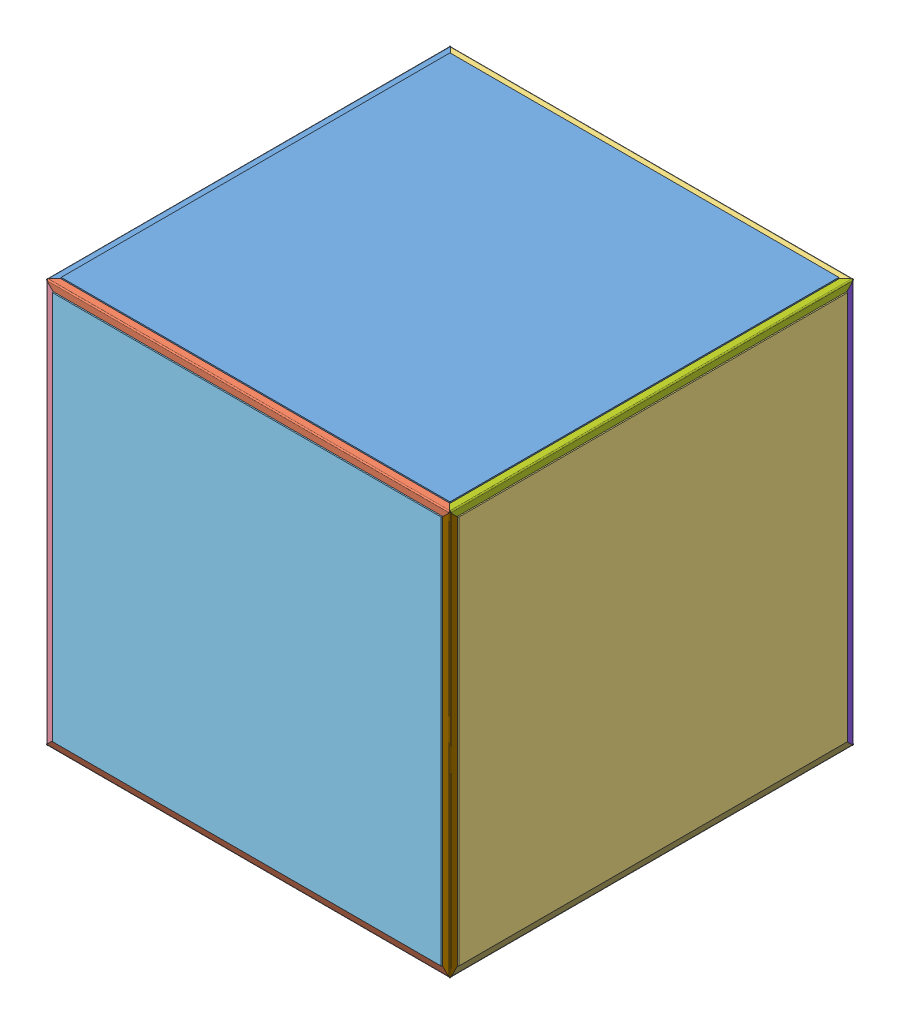
SolidWorks assembly cube_32, configuration cube32. Lengths in mm.
Overall size (513.72 513.72 513.72).
30 component instances, 30 part files, 93 mates.
Components (placement in the parent):
- pr^cube_32-28: pr^cube_32 [cube01] x (-1 0 0) z (0 0 1) size (491.49 1.59 491.49) (virtual)
- pg^cube_32-20: pg^cube_32 [cube01] x (0 -1 0) z (0 0 1) size (491.49 1.59 491.49) (virtual)
- po^cube_32-22: po^cube_32 [cube01] x (0 1 0) z (0 0 1) size (491.49 1.59 491.49) (virtual)
- py^cube_32-21: py^cube_32 [cube01] at origin size (491.49 1.59 491.49) (virtual)
- pc^cube_32-18: pc^cube_32 [cube01] x (-1 0 0) z (0 -1 0) size (491.49 1.59 491.49) (virtual)
- pb^cube_32-21: pb^cube_32 [cube01] x (-1 0 0) z (0 1 0) size (491.49 1.59 491.49) (virtual)
- br1^cube_32-49: br1^cube_32 [Default] at (0 229.87 -229.87) x (0 0 1) z (-1 0 0) size (50.8 50.8 452.63) (virtual)
- br2^cube_32-61: br2^cube_32 [Default] at (-229.87 229.87 0) size (50.8 50.8 452.63) (virtual)
- br3^cube_32-46: br3^cube_32 [Default] at (0 229.87 229.87) x (0 0 -1) z (1 0 0) size (50.8 50.8 452.63) (virtual)
- bg1^cube_32-47: bg1^cube_32 [Default] at (-229.87 -229.87 0) x (0 1 0) z (0 0 1) size (50.8 50.8 452.63) (virtual)
- bg2^cube_32-44: bg2^cube_32 [Default] at (-229.87 0 229.87) x (0 0 -1) z (0 1 0) size (50.8 50.8 452.63) (virtual)
- bg3^cube_32-40: bg3^cube_32 [Default] at (-229.87 0 -229.87) x (0 0 1) z (0 -1 0) size (50.8 50.8 452.63) (virtual)
- bo1^cube_32-42: bo1^cube_32 [Default] at (229.87 0 -229.87) x (0 0 1) z (0 1 0) size (50.8 50.8 452.63) (virtual)
- bo2^cube_32-46: bo2^cube_32 [Default] at (229.87 0 229.87) x (0 0 -1) z (0 -1 0) size (50.8 50.8 452.63) (virtual)
- bo3^cube_32-62: bo3^cube_32 [Default] at (229.87 229.87 0) x (0 -1 0) z (0 0 1) size (50.8 50.8 452.63) (virtual)
- by1^cube_32-41: by1^cube_32 [Default] at (0 -229.87 -229.87) x (0 0 1) z (1 0 0) size (50.8 50.8 452.63) (virtual)
- by2^cube_32-45: by2^cube_32 [Default] at (0 -229.87 229.87) x (0 0 -1) z (-1 0 0) size (50.8 50.8 452.63) (virtual)
- by3^cube_32-48: by3^cube_32 [Default] at (229.87 -229.87 0) x (-1 0 0) z (0 0 1) size (50.8 50.8 452.63) (virtual)
- dr1^cube_32-55: dr1^cube_32 [cube01] at (-254.6646 255.27 0) x (0 -1 0) z (0 0 1) size (26.01 26.01 510.55) (hidden, virtual)
- dr2^cube_32-37: dr2^cube_32 [cube01] at (0 255.27 254.6646) x (0 -1 0) z (1 0 0) size (26.01 26.01 510.55) (hidden, virtual)
- dr3^cube_32-33: dr3^cube_32 [cube01] at (0 255.27 -254.6646) x (0 -1 0) z (-1 0 0) size (26.01 26.01 510.55) (hidden, virtual)
- dg1^cube_32-38: dg1^cube_32 [cube01] at (-255.27 0 254.6646) x (1 0 0) z (0 1 0) size (26.01 26.01 510.55) (hidden, virtual)
- dg2^cube_32-41: dg2^cube_32 [cube01] at (-255.27 -254.6646 0) size (26.01 26.01 510.55) (hidden, virtual)
- dg3^cube_32-34: dg3^cube_32 [cube01] at (-255.27 0 -254.6646) x (1 0 0) z (0 -1 0) size (26.01 26.01 510.55) (hidden, virtual)
- do3^cube_32-47: do3^cube_32 [cube01] at (255.27 254.6646 0) x (-1 0 0) z (0 0 1) size (26.01 26.01 510.55) (hidden, virtual)
- do1^cube_32-36: do1^cube_32 [cube01] at (255.27 0 -254.6646) x (-1 0 0) z (0 1 0) size (26.01 26.01 510.55) (hidden, virtual)
- do2^cube_32-40: do2^cube_32 [cube01] at (255.27 0 254.6646) x (-1 0 0) z (0 -1 0) size (26.01 26.01 510.55) (hidden, virtual)
- dy1^cube_32-35: dy1^cube_32 [cube01] at (0 -255.27 -254.6646) x (0 1 0) z (1 0 0) size (26.01 26.01 510.55) (hidden, virtual)
- dy2^cube_32-39: dy2^cube_32 [cube01] at (0 -255.27 254.6646) x (0 1 0) z (-1 0 0) size (26.01 26.01 510.55) (hidden, virtual)
- dy3^cube_32-42: dy3^cube_32 [cube01] at (254.6646 -255.27 0) x (0 1 0) z (0 0 1) size (26.01 26.01 510.55) (hidden, virtual)
Mates (geometry in assembly coordinates):
- Coincident1: coincident anti-aligned: plane of pr^cube_32-28 through (245.745 255.27 -245.745) normal (0 -1 0); plane of br1^cube_32-49 through (-226.314 255.27 -229.87) normal (0 1 0)
- Coincident2: coincident anti-aligned: plane of pr^cube_32-28 through (245.745 255.27 -245.745) normal (0 -1 0); plane of br2^cube_32-61 through (-229.87 255.27 226.314) normal (0 1 0)
- Coincident3: coincident anti-aligned: plane of pr^cube_32-28 through (245.745 255.27 -245.745) normal (0 -1 0); plane of br3^cube_32-46 through (226.314 255.27 229.87) normal (0 1 0)
- Coincident4: coincident anti-aligned: plane of pr^cube_32-28 through (245.745 255.27 -245.745) normal (0 -1 0); plane of bo3^cube_32-62 through (229.87 255.27 226.314) normal (0 1 0)
- Coincident5: coincident anti-aligned: plane of pr^cube_32-28 through (245.745 255.27 -245.745) normal (0 -1 0); plane of dr3^cube_32-33 through (0 255.27 -509.9346) normal (0 1 0)
- Coincident6: coincident anti-aligned: plane of pr^cube_32-28 through (245.745 255.27 -245.745) normal (0 -1 0); plane of dr1^cube_32-55 through (-509.9346 255.27 0) normal (0 1 0)
- Coincident7: coincident anti-aligned: plane of pr^cube_32-28 through (245.745 255.27 -245.745) normal (0 -1 0); plane of do3^cube_32-47 through (-0.6054 255.27 0) normal (0 1 0)
- Coincident8: coincident anti-aligned: plane of pr^cube_32-28 through (245.745 255.27 -245.745) normal (0 -1 0); plane of dr2^cube_32-37 through (0 255.27 509.9346) normal (0 1 0)
- Coincident34: coincident anti-aligned: plane of pb^cube_32-21 through (245.745 -245.745 -255.27) normal (0 0 1); plane of by1^cube_32-41 through (226.314 -229.87 -255.27) normal (0 0 -1)
- Coincident35: coincident anti-aligned: plane of pb^cube_32-21 through (245.745 -245.745 -255.27) normal (0 0 1); plane of bo1^cube_32-42 through (229.87 226.314 -255.27) normal (0 0 -1)
- Coincident36: coincident anti-aligned: plane of pb^cube_32-21 through (245.745 -245.745 -255.27) normal (0 0 1); plane of br1^cube_32-49 through (-226.314 229.87 -255.27) normal (0 0 -1)
- Coincident37: coincident anti-aligned: plane of pb^cube_32-21 through (245.745 -245.745 -255.27) normal (0 0 1); plane of bg3^cube_32-40 through (-229.87 -226.314 -255.27) normal (0 0 -1)
- Coincident38: coincident anti-aligned: plane of pb^cube_32-21 through (245.745 -245.745 -255.27) normal (0 0 1); plane of dg3^cube_32-34 through (0.6054 0 -255.27) normal (0 0 -1)
- Coincident39: coincident anti-aligned: plane of pb^cube_32-21 through (245.745 -245.745 -255.27) normal (0 0 1); plane of dr3^cube_32-33 through (0 -0.6054 -255.27) normal (0 0 -1)
- Coincident40: coincident anti-aligned: plane of pb^cube_32-21 through (245.745 -245.745 -255.27) normal (0 0 1); plane of do1^cube_32-36 through (-0.6054 0 -255.27) normal (0 0 -1)
- Coincident41: coincident anti-aligned: plane of pb^cube_32-21 through (245.745 -245.745 -255.27) normal (0 0 1); plane of dy1^cube_32-35 through (0 0.6054 -255.27) normal (0 0 -1)
- Coincident42: coincident anti-aligned: plane of pc^cube_32-18 through (245.745 245.745 255.27) normal (0 0 -1); plane of bo2^cube_32-46 through (229.87 -226.314 255.27) normal (0 0 1)
- Coincident43: coincident anti-aligned: plane of pc^cube_32-18 through (245.745 245.745 255.27) normal (0 0 -1); plane of br3^cube_32-46 through (226.314 229.87 255.27) normal (0 0 1)
- Coincident44: coincident anti-aligned: plane of pc^cube_32-18 through (245.745 245.745 255.27) normal (0 0 -1); plane of bg2^cube_32-44 through (-229.87 226.314 255.27) normal (0 0 1)
- Coincident45: coincident anti-aligned: plane of pc^cube_32-18 through (245.745 245.745 255.27) normal (0 0 -1); plane of by2^cube_32-45 through (-226.314 -229.87 255.27) normal (0 0 1)
- Coincident46: coincident anti-aligned: plane of pc^cube_32-18 through (245.745 245.745 255.27) normal (0 0 -1); plane of do2^cube_32-40 through (-0.6054 0 255.27) normal (0 0 1)
- Coincident47: coincident anti-aligned: plane of pc^cube_32-18 through (245.745 245.745 255.27) normal (0 0 -1); plane of dy2^cube_32-39 through (0 0.6054 255.27) normal (0 0 1)
- Coincident48: coincident anti-aligned: plane of pc^cube_32-18 through (245.745 245.745 255.27) normal (0 0 -1); plane of dg1^cube_32-38 through (0.6054 0 255.27) normal (0 0 1)
- Coincident49: coincident anti-aligned: plane of pc^cube_32-18 through (245.745 245.745 255.27) normal (0 0 -1); plane of dr2^cube_32-37 through (0 -0.6054 255.27) normal (0 0 1)
- Coincident50: coincident anti-aligned: plane of pg^cube_32-20 through (-255.27 245.745 -245.745) normal (1 0 0); plane of bg3^cube_32-40 through (-255.27 -226.314 -229.87) normal (-1 0 0)
- Coincident51: coincident anti-aligned: plane of pg^cube_32-20 through (-255.27 245.745 -245.745) normal (1 0 0); plane of bg1^cube_32-47 through (-255.27 -229.87 226.314) normal (-1 0 0)
- Coincident52: coincident anti-aligned: plane of pg^cube_32-20 through (-255.27 245.745 -245.745) normal (1 0 0); plane of bg2^cube_32-44 through (-255.27 226.314 229.87) normal (-1 0 0)
- Coincident53: coincident anti-aligned: plane of pg^cube_32-20 through (-255.27 245.745 -245.745) normal (1 0 0); plane of dr1^cube_32-55 through (-255.27 -0.6054 0) normal (-1 0 0)
- Coincident54: coincident anti-aligned: plane of pg^cube_32-20 through (-255.27 245.745 -245.745) normal (1 0 0); plane of dg3^cube_32-34 through (-255.27 0 -509.9346) normal (-1 0 0)
- Coincident55: coincident anti-aligned: plane of pg^cube_32-20 through (-255.27 245.745 -245.745) normal (1 0 0); plane of dg2^cube_32-41 through (-255.27 -509.9346 0) normal (-1 0 0)
- Coincident56: coincident anti-aligned: plane of pg^cube_32-20 through (-255.27 245.745 -245.745) normal (1 0 0); plane of dg1^cube_32-38 through (-255.27 0 509.9346) normal (-1 0 0)
- Coincident99: coincident anti-aligned: plane of pg^cube_32-20 through (-255.27 245.745 -245.745) normal (1 0 0); plane of br2^cube_32-61 through (-255.27 229.87 226.314) normal (-1 0 0)
- Coincident57: coincident anti-aligned: plane of py^cube_32-21 through (-245.745 -255.27 -245.745) normal (0 1 0); plane of by3^cube_32-48 through (229.87 -255.27 226.314) normal (0 -1 0)
- Coincident58: coincident anti-aligned: plane of py^cube_32-21 through (-245.745 -255.27 -245.745) normal (0 1 0); plane of by2^cube_32-45 through (-226.314 -255.27 229.87) normal (0 -1 0)
- Coincident59: coincident anti-aligned: plane of py^cube_32-21 through (-245.745 -255.27 -245.745) normal (0 1 0); plane of bg1^cube_32-47 through (-229.87 -255.27 226.314) normal (0 -1 0)
- Coincident60: coincident anti-aligned: plane of py^cube_32-21 through (-245.745 -255.27 -245.745) normal (0 1 0); plane of by1^cube_32-41 through (226.314 -255.27 -229.87) normal (0 -1 0)
- Coincident61: coincident anti-aligned: plane of py^cube_32-21 through (-245.745 -255.27 -245.745) normal (0 1 0); plane of dy3^cube_32-42 through (509.9346 -255.27 0) normal (0 -1 0)
- Coincident62: coincident anti-aligned: plane of py^cube_32-21 through (-245.745 -255.27 -245.745) normal (0 1 0); plane of dy2^cube_32-39 through (0 -255.27 509.9346) normal (0 -1 0)
- Coincident63: coincident anti-aligned: plane of py^cube_32-21 through (-245.745 -255.27 -245.745) normal (0 1 0); plane of dg2^cube_32-41 through (0.6054 -255.27 0) normal (0 -1 0)
- Coincident64: coincident anti-aligned: plane of py^cube_32-21 through (-245.745 -255.27 -245.745) normal (0 1 0); plane of dy1^cube_32-35 through (0 -255.27 -509.9346) normal (0 -1 0)
- Coincident65: coincident anti-aligned: plane of po^cube_32-22 through (255.27 -245.745 -245.745) normal (-1 0 0); plane of bo1^cube_32-42 through (255.27 226.314 -229.87) normal (1 0 0)
- Coincident66: coincident anti-aligned: plane of po^cube_32-22 through (255.27 -245.745 -245.745) normal (-1 0 0); plane of by3^cube_32-48 through (255.27 -229.87 226.314) normal (1 0 0)
- Coincident67: coincident anti-aligned: plane of po^cube_32-22 through (255.27 -245.745 -245.745) normal (-1 0 0); plane of bo2^cube_32-46 through (255.27 -226.314 229.87) normal (1 0 0)
- Coincident68: coincident anti-aligned: plane of po^cube_32-22 through (255.27 -245.745 -245.745) normal (-1 0 0); plane of bo3^cube_32-62 through (255.27 229.87 226.314) normal (1 0 0)
- Coincident69: coincident anti-aligned: plane of po^cube_32-22 through (255.27 -245.745 -245.745) normal (-1 0 0); plane of do2^cube_32-40 through (255.27 0 509.9346) normal (1 0 0)
- Coincident70: coincident anti-aligned: plane of po^cube_32-22 through (255.27 -245.745 -245.745) normal (-1 0 0); plane of do3^cube_32-47 through (255.27 509.9346 0) normal (1 0 0)
- Coincident71: coincident anti-aligned: plane of po^cube_32-22 through (255.27 -245.745 -245.745) normal (-1 0 0); plane of do1^cube_32-36 through (255.27 0 -509.9346) normal (1 0 0)
- Coincident72: coincident anti-aligned: plane of po^cube_32-22 through (255.27 -245.745 -245.745) normal (-1 0 0); plane of dy3^cube_32-42 through (255.27 0.6054 0) normal (1 0 0)
- Coincident73: coincident aligned: plane of assembly through (0 0 0) normal (0 0 1); plane of dy3^cube_32-42 through (254.6646 -255.27 0) normal (0 0 1)
- Coincident74: coincident aligned: plane of assembly through (0 0 0) normal (0 0 1); plane of by3^cube_32-48 through (229.87 -229.87 0) normal (0 0 1)
- Coincident75: coincident aligned: plane of assembly through (0 0 0) normal (0 0 1); plane of bo3^cube_32-62 through (229.87 229.87 0) normal (0 0 1)
- Coincident76: coincident aligned: plane of assembly through (0 0 0) normal (0 0 1); plane of do3^cube_32-47 through (255.27 254.6646 0) normal (0 0 1)
- Coincident77: coincident aligned: plane of assembly through (0 0 0) normal (0 0 1); plane of dg2^cube_32-41 through (-255.27 -254.6646 0) normal (0 0 1)
- Coincident78: coincident aligned: plane of assembly through (0 0 0) normal (0 0 1); plane of bg1^cube_32-47 through (-229.87 -229.87 0) normal (0 0 1)
- Coincident79: coincident aligned: plane of assembly through (0 0 0) normal (0 0 1); plane of dr1^cube_32-55 through (-254.6646 255.27 0) normal (0 0 1)
- Coincident80: coincident aligned: plane of assembly through (0 0 0) normal (0 0 1); plane of br2^cube_32-61 through (-229.87 229.87 0) normal (0 0 1)
- Coincident81: coincident aligned: plane of assembly through (0 0 0) normal (0 1 0); plane of bo1^cube_32-42 through (229.87 0 -229.87) normal (0 1 0)
- Coincident82: coincident aligned: plane of assembly through (0 0 0) normal (0 1 0); plane of py^cube_32-21 through (0 0 0) normal (0 1 0)
- Coincident83: coincident aligned: plane of assembly through (0 0 0) normal (0 1 0); plane of do1^cube_32-36 through (255.27 0 -254.6646) normal (0 1 0)
- Coincident84: coincident anti-aligned: plane of assembly through (0 0 0) normal (0 1 0); plane of bg3^cube_32-40 through (-229.87 0 -229.87) normal (0 -1 0)
- Coincident85: coincident anti-aligned: plane of assembly through (0 0 0) normal (0 1 0); plane of dg3^cube_32-34 through (-255.27 0 -254.6646) normal (0 -1 0)
- Coincident86: coincident aligned: plane of assembly through (0 0 0) normal (0 1 0); plane of dg1^cube_32-38 through (-255.27 0 254.6646) normal (0 1 0)
- Coincident87: coincident aligned: plane of assembly through (0 0 0) normal (0 1 0); plane of bg2^cube_32-44 through (-229.87 0 229.87) normal (0 1 0)
- Coincident88: coincident anti-aligned: plane of assembly through (0 0 0) normal (0 1 0); plane of bo2^cube_32-46 through (229.87 0 229.87) normal (0 -1 0)
- Coincident89: coincident anti-aligned: plane of assembly through (0 0 0) normal (0 1 0); plane of do2^cube_32-40 through (255.27 0 254.6646) normal (0 -1 0)
- Coincident90: coincident anti-aligned: plane of assembly through (0 0 0) normal (1 0 0); plane of by2^cube_32-45 through (0 -229.87 229.87) normal (-1 0 0)
- Coincident91: coincident anti-aligned: plane of assembly through (0 0 0) normal (1 0 0); plane of dy2^cube_32-39 through (0 -255.27 254.6646) normal (-1 0 0)
- Coincident92: coincident aligned: plane of assembly through (0 0 0) normal (1 0 0); plane of pg^cube_32-20
- Coincident93: coincident aligned: plane of assembly through (0 0 0) normal (1 0 0); plane of dr2^cube_32-37 through (0 255.27 254.6646) normal (1 0 0)
- Coincident94: coincident aligned: plane of assembly through (0 0 0) normal (1 0 0); plane of br3^cube_32-46 through (0 229.87 229.87) normal (1 0 0)
- Coincident95: coincident anti-aligned: plane of assembly through (0 0 0) normal (1 0 0); plane of dr3^cube_32-33 through (0 255.27 -254.6646) normal (-1 0 0)
- Coincident96: coincident anti-aligned: plane of assembly through (0 0 0) normal (1 0 0); plane of br1^cube_32-49 through (0 229.87 -229.87) normal (-1 0 0)
- Coincident97: coincident aligned: plane of assembly through (0 0 0) normal (1 0 0); plane of by1^cube_32-41 through (0 -229.87 -229.87) normal (1 0 0)
- Coincident98: coincident aligned: plane of assembly through (0 0 0) normal (1 0 0); plane of dy1^cube_32-35 through (0 -255.27 -254.6646) normal (1 0 0)
- Coincident100: coincident anti-aligned: plane of pr^cube_32-28; plane of assembly through (0 0 0) normal (1 0 0)
- Coincident101: coincident aligned: plane of pr^cube_32-28 through (0 0 0) normal (0 0 1); plane of assembly through (0 0 0) normal (0 0 1)
- Coincident102: coincident anti-aligned: plane of pr^cube_32-28; plane of assembly through (0 0 0) normal (0 1 0)
- Coincident106: coincident anti-aligned: plane of pg^cube_32-20; plane of assembly through (0 0 0) normal (0 1 0)
- Coincident107: coincident aligned: plane of pg^cube_32-20; plane of assembly through (0 0 0) normal (1 0 0)
- Coincident108: coincident aligned: plane of pg^cube_32-20 through (0 0 0) normal (0 0 1); plane of assembly through (0 0 0) normal (0 0 1)
- Coincident109: coincident aligned: plane of py^cube_32-21 through (0 0 0) normal (0 0 1); plane of assembly through (0 0 0) normal (0 0 1)
- Coincident110: coincident aligned: plane of py^cube_32-21 through (0 0 0) normal (0 1 0); plane of assembly through (0 0 0) normal (0 1 0)
- Coincident111: coincident aligned: plane of py^cube_32-21 through (0 0 0) normal (1 0 0); plane of assembly through (0 0 0) normal (1 0 0)
- Coincident112: coincident aligned: plane of po^cube_32-22 through (0 0 0) normal (0 0 1); plane of assembly through (0 0 0) normal (0 0 1)
- Coincident113: coincident anti-aligned: plane of po^cube_32-22; plane of assembly through (0 0 0) normal (1 0 0)
- Coincident114: coincident aligned: plane of po^cube_32-22; plane of assembly through (0 0 0) normal (0 1 0)
- Coincident115: coincident anti-aligned: plane of pc^cube_32-18 through (0 0 0) normal (0 -1 0); plane of assembly through (0 0 0) normal (0 1 0)
- Coincident116: coincident anti-aligned: plane of pc^cube_32-18; plane of assembly through (0 0 0) normal (0 0 1)
- Coincident117: coincident anti-aligned: plane of pc^cube_32-18; plane of assembly through (0 0 0) normal (1 0 0)
- Coincident118: coincident aligned: plane of pb^cube_32-21 through (0 0 0) normal (0 1 0); plane of assembly through (0 0 0) normal (0 1 0)
- Coincident119: coincident aligned: plane of pb^cube_32-21; plane of assembly through (0 0 0) normal (0 0 1)
- Coincident120: coincident anti-aligned: line of pb^cube_32-21 through (0.8731 -0.8731 0) axis (0 0 -1); sketch_entity of pr^cube_32-28; plane of pb^cube_32-21 through (245.745 -245.745 -256.8575) normal (0 0 -1); plane of py^cube_32-21 through (-245.745 -256.8575 -245.745) normal (0 -1 0)
- cyan_cut: unknown: unknown of pc^cube_32-18; plane of pc^cube_32-18 through (245.745 245.745 256.8575) normal (0 0 1); plane of pg^cube_32-20 through (-256.8575 245.745 -245.745) normal (-1 0 0); plane of po^cube_32-22 through (256.8575 -245.745 -245.745) normal (1 0 0)
